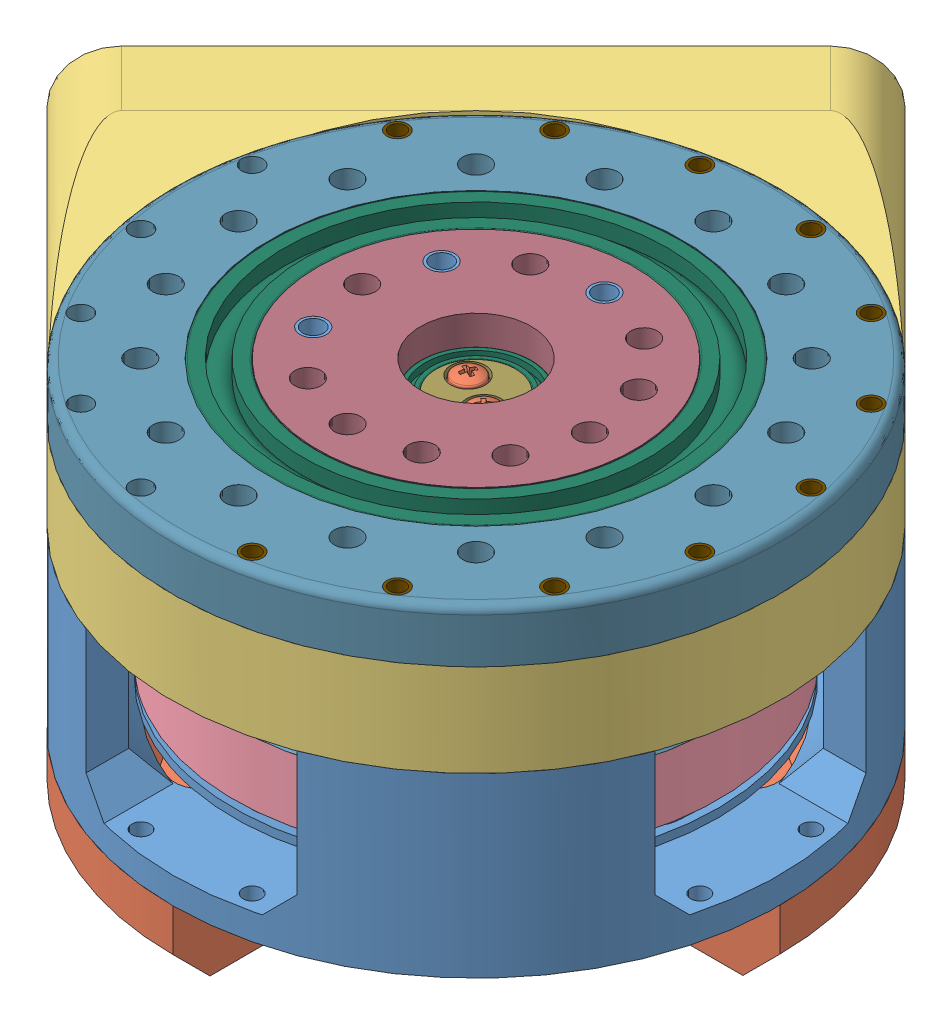
SolidWorks assembly Cycloidal_v2, configuration Default. Lengths in mm.
Overall size (173.24 87.5 173.24).
352 component instances, 93 part files, 142 mates.
Components (placement in the parent):
- motor-X83008S.stp-1: motor-X83008S.stp [Default] at (84.8609 89.8915 111.5645) x (-0.966627 0 -0.256188) z (0 -1 0) size (114.7 114.7 37.62)
  - base.stp-1: base.stp [Default] at (42.0794 12.0269 46.7342) size (91.6 91.6 15.61)
  - stator.stp-1: stator.stp [Default] at (42.0794 12.0269 33.1342) x (0.08493 -0.996387 0) z (0 0 1) size (83 83 8)
  - coil.stp-1: coil.stp [Default] at (39.5332 41.8984 37.1342) x (0.996387 0.08493 0) z (-0.08493 0.996387 0) size (4.4 10.2 10.5)
  - coil.stp-2: coil.stp [Default] at (34.3848 41.0025 37.1342) x (0.966502 0.256661 0) z (-0.256661 0.966502 0) size (4.4 10.2 10.5)
  - coil.stp-3: coil.stp [Default] at (29.4701 39.2261 37.1342) x (0.90725 0.420593 0) z (-0.420593 0.90725 0) size (4.4 10.2 10.5)
  - coil.stp-4: coil.stp [Default] at (24.9386 36.6233 37.1342) x (0.820431 0.571745 0) z (-0.571745 0.820431 0) size (4.4 10.2 10.5)
  - coil.stp-5: coil.stp [Default] at (20.9279 33.2732 37.1342) x (0.708685 0.705525 0) z (-0.705525 0.708685 0) size (4.4 10.2 10.5)
  - coil.stp-6: coil.stp [Default] at (17.5599 29.2775 37.1342) x (0.575405 0.817869 0) z (-0.817869 0.575405 0) size (4.4 10.2 10.5)
  - coil.stp-7: coil.stp [Default] at (14.9368 24.7576 37.1342) x (0.424642 0.905361 0) z (-0.905361 0.424642 0) size (4.4 10.2 10.5)
  - coil.stp-8: coil.stp [Default] at (13.1385 19.8509 37.1342) x (0.260976 0.965345 0) z (-0.965345 0.260976 0) size (4.4 10.2 10.5)
  - coil.stp-9: coil.stp [Default] at (12.2196 14.7066 37.1342) x (0.089381 0.995998 0) z (-0.995998 0.089381 0) size (4.4 10.2 10.5)
  - coil.stp-10: coil.stp [Default] at (12.2079 9.4807 37.1342) x (-0.08493 0.996387 0) z (-0.996387 -0.08493 0) size (4.4 10.2 10.5)
  - coil.stp-11: coil.stp [Default] at (13.1039 4.3323 37.1342) x (-0.256661 0.966502 0) z (-0.966502 -0.256661 0) size (4.4 10.2 10.5)
  - coil.stp-12: coil.stp [Default] at (14.8802 -0.5824 37.1342) x (-0.420593 0.90725 0) z (-0.90725 -0.420593 0) size (4.4 10.2 10.5)
  - coil.stp-13: coil.stp [Default] at (17.483 -5.1139 37.1342) x (-0.571745 0.820431 0) z (-0.820431 -0.571745 0) size (4.4 10.2 10.5)
  - coil.stp-14: coil.stp [Default] at (20.8332 -9.1246 37.1342) x (-0.705525 0.708685 0) z (-0.708685 -0.705525 0) size (4.4 10.2 10.5)
  - coil.stp-15: coil.stp [Default] at (24.8289 -12.4926 37.1342) x (-0.817869 0.575405 0) z (-0.575405 -0.817869 0) size (4.4 10.2 10.5)
  - coil.stp-16: coil.stp [Default] at (29.3487 -15.1157 37.1342) x (-0.905361 0.424642 0) z (-0.424642 -0.905361 0) size (4.4 10.2 10.5)
  - coil.stp-17: coil.stp [Default] at (34.2554 -16.914 37.1342) x (-0.965345 0.260976 0) z (-0.260976 -0.965345 0) size (4.4 10.2 10.5)
  - coil.stp-18: coil.stp [Default] at (39.3998 -17.8329 37.1342) x (-0.995998 0.089381 0) z (-0.089381 -0.995998 0) size (4.4 10.2 10.5)
  - coil.stp-19: coil.stp [Default] at (44.6256 -17.8446 37.1342) x (-0.996387 -0.08493 0) z (0.08493 -0.996387 0) size (4.4 10.2 10.5)
  - coil.stp-20: coil.stp [Default] at (49.7741 -16.9486 37.1342) x (-0.966502 -0.256661 0) z (0.256661 -0.966502 0) size (4.4 10.2 10.5)
  - coil.stp-21: coil.stp [Default] at (54.6887 -15.1723 37.1342) x (-0.90725 -0.420593 0) z (0.420593 -0.90725 0) size (4.4 10.2 10.5)
  - coil.stp-22: coil.stp [Default] at (59.2202 -12.5695 37.1342) x (-0.820431 -0.571745 0) z (0.571745 -0.820431 0) size (4.4 10.2 10.5)
  - coil.stp-23: coil.stp [Default] at (63.2309 -9.2193 37.1342) x (-0.708685 -0.705525 0) z (0.705525 -0.708685 0) size (4.4 10.2 10.5)
  - coil.stp-24: coil.stp [Default] at (66.599 -5.2236 37.1342) x (-0.575405 -0.817869 0) z (0.817869 -0.575405 0) size (4.4 10.2 10.5)
  - coil.stp-25: coil.stp [Default] at (69.222 -0.7038 37.1342) x (-0.424642 -0.905361 0) z (0.905361 -0.424642 0) size (4.4 10.2 10.5)
  - coil.stp-26: coil.stp [Default] at (71.0203 4.2029 37.1342) x (-0.260976 -0.965345 0) z (0.965345 -0.260976 0) size (4.4 10.2 10.5)
  - coil.stp-27: coil.stp [Default] at (71.9392 9.3473 37.1342) x (-0.089381 -0.995998 0) z (0.995998 -0.089381 0) size (4.4 10.2 10.5)
  - coil.stp-28: coil.stp [Default] at (71.9509 14.5731 37.1342) x (0.08493 -0.996387 0) z (0.996387 0.08493 0) size (4.4 10.2 10.5)
  - coil.stp-29: coil.stp [Default] at (71.055 19.7216 37.1342) x (0.256661 -0.966502 0) z (0.966502 0.256661 0) size (4.4 10.2 10.5)
  - coil.stp-30: coil.stp [Default] at (69.2786 24.6362 37.1342) x (0.420593 -0.90725 0) z (0.90725 0.420593 0) size (4.4 10.2 10.5)
  - coil.stp-31: coil.stp [Default] at (66.6758 29.1677 37.1342) x (0.571745 -0.820431 0) z (0.820431 0.571745 0) size (4.4 10.2 10.5)
  - coil.stp-32: coil.stp [Default] at (63.3257 33.1785 37.1342) x (0.705525 -0.708685 0) z (0.708685 0.705525 0) size (4.4 10.2 10.5)
  - coil.stp-33: coil.stp [Default] at (59.33 36.5465 37.1342) x (0.817869 -0.575405 0) z (0.575405 0.817869 0) size (4.4 10.2 10.5)
  - coil.stp-34: coil.stp [Default] at (54.8101 39.1695 37.1342) x (0.905361 -0.424642 0) z (0.424642 0.905361 0) size (4.4 10.2 10.5)
  - coil.stp-35: coil.stp [Default] at (49.9034 40.9678 37.1342) x (0.965345 -0.260976 0) z (0.260976 0.965345 0) size (4.4 10.2 10.5)
  - coil.stp-36: coil.stp [Default] at (44.759 41.8868 37.1342) x (0.995998 -0.089381 0) z (0.089381 0.995998 0) size (4.4 10.2 10.5)
  - rotor.stp-1: rotor.stp [Default] at (42.0794 12.0269 42.1342) x (-0.293442 0.955977 0) z (0 0 -1) size (91.8 91.8 12)
  - outrunner.stp-1: outrunner.stp [Default] at (42.0794 12.0269 30.1342) x (-0.254711 0.967017 0) z (-0.967017 -0.254711 0) size (91.8 17.01 91.8)
  - screw-mount.stp-1: screw-mount.stp [Default] at (38.1314 27.0157 27.1342) x (1 0 0) z (0 0 -1) size (7 7 6.5)
  - screw-mount.stp-2: screw-mount.stp [Default] at (27.0906 8.0789 27.1342) x (1 0 0) z (0 0 -1) size (7 7 6.5)
  - screw-mount.stp-3: screw-mount.stp [Default] at (57.0682 15.9749 27.1342) x (1 0 0) z (0 0 -1) size (7 7 6.5)
  - screw-mount.stp-4: screw-mount.stp [Default] at (46.0274 -2.9618 27.1342) x (1 0 0) z (0 0 -1) size (7 7 6.5)
  - 6702ZZ-bearing-15x21x4.stp-1: 6702ZZ-bearing-15x21x4.stp [Default] at (42.0794 12.0269 43.7342) x (1 0 0) z (0 -1 0) size (21 4 21)
  - 6702ZZ-bearing-15x21x4.stp-2: 6702ZZ-bearing-15x21x4.stp [Default] at (42.0794 12.0269 35.1342) x (1 0 0) z (0 1 0) size (21 4 21)
  - shaft.stp-1: shaft.stp [Default] at (42.0794 12.0269 20.1342) size (16 16 31.6)
  - fix-screw.stp-1: fix-screw.stp [Default] at (42.0794 12.0269 51.7342) x (1 0 0) z (0 0 -1) size (19.67 18.96 12.02)
- Base_Plate-1: Base_Plate [Default] at (47.267 69.7573 89.1587) x (0.869491 0 0.493949) z (-0.493949 0 0.869491) size (40 7 40)
- Eccentric_Shaft-1: Eccentric_Shaft [Default] at (31.2466 70.4165 88.8331) x (0.493949 0 -0.869491) z (0.869491 0 0.493949) size (20 15 17)
  - Eccentric_Shaft_bot-1: Eccentric_Shaft_bot [Default] at (7.6302 6.3409 14.0904) size (17 5 17)
  - Eccentric_Shaft_bot-2: Eccentric_Shaft_bot [Default] at (7.6302 11.3409 14.0904) x (-1 0 0) z (0 0 -1) size (17 5 17)
  - Eccentric_Shaft_top-1: Eccentric_Shaft_top [Default] at (7.6302 16.3409 14.0904) x (-1 0 0) z (0 0 -1) size (17 5 17)
- Output_Shaft-1: Output_Shaft [Default] at (47.267 87.2573 89.1587) x (-0.447203 0 -0.894433) z (0.894433 0 -0.447203) size (60 10 60)
- Cover-1: Cover [Default] at (47.267 87.2573 89.1587) x (0.707107 0 -0.707107) z (0.707107 0 0.707107) size (115 10.4 115)
- radial ball bearing_68_iso-39: radial ball bearing_68_iso [ISO 15 RBB - 1860 - 32,SI,NC,32_68] at (47.267 92.2573 89.1587) x (0 1 0) z (0 0 1) size (10 78 78)
- radial ball bearing_68_iso-40: radial ball bearing_68_iso [ISO 15 RBB - 1840 - 32,SI,NC,32_68] at (47.267 73.2573 89.1587) x (0 1 0) z (-0.019534 0 0.999809) size (7 52 52)
- m13_bearing-31: m13_bearing [Default] at (-10.7414 95.4081 67.0593) x (0.227678 0 0.973736) z (0.973736 0 -0.227678) size (13 16 13)
  - m6-1: m6 [Default] at (8.4921 2.5508 14.8914) size (6 16 6)
  - radial ball bearing_68_iso-1: radial ball bearing_68_iso [ISO 15 RBB - 286 - 10,SI,NC,10_68] at (8.4921 16.0508 14.8914) x (0 1 0) z (0 0 1) size (5 13 13)
  - radial ball bearing_68_iso-2: radial ball bearing_68_iso [ISO 15 RBB - 286 - 10,SI,NC,10_68] at (8.4921 11.0508 14.8914) x (0 1 0) z (0 0 1) size (5 13 13)
- m13_bearing-32: m13_bearing [Default] at (-14.1668 95.4081 84.2801) x (0.227678 0 0.973736) z (0.973736 0 -0.227678) size (13 16 13)
  - m6-1: m6 [Default] at (8.4921 2.5508 14.8914) size (6 16 6)
  - radial ball bearing_68_iso-1: radial ball bearing_68_iso [ISO 15 RBB - 286 - 10,SI,NC,10_68] at (8.4921 16.0508 14.8914) x (0 1 0) z (0 0 1) size (5 13 13)
  - radial ball bearing_68_iso-2: radial ball bearing_68_iso [ISO 15 RBB - 286 - 10,SI,NC,10_68] at (8.4921 11.0508 14.8914) x (0 1 0) z (0 0 1) size (5 13 13)
- m13_bearing-34: m13_bearing [Default] at (13.6125 95.5581 125.8547) x (0.227678 0 0.973736) z (0.973736 0 -0.227678) size (13 16 13)
  - m6-1: m6 [Default] at (8.4921 2.5508 14.8914) size (6 16 6)
  - radial ball bearing_68_iso-1: radial ball bearing_68_iso [ISO 15 RBB - 286 - 10,SI,NC,10_68] at (8.4921 16.0508 14.8914) x (0 1 0) z (0 0 1) size (5 13 13)
  - radial ball bearing_68_iso-2: radial ball bearing_68_iso [ISO 15 RBB - 286 - 10,SI,NC,10_68] at (8.4921 11.0508 14.8914) x (0 1 0) z (0 0 1) size (5 13 13)
- m13_bearing-35: m13_bearing [Default] at (-0.9866 95.4081 116.0999) x (0.227678 0 0.973736) z (0.973736 0 -0.227678) size (13 16 13)
  - m6-1: m6 [Default] at (8.4921 2.5508 14.8914) size (6 16 6)
  - radial ball bearing_68_iso-1: radial ball bearing_68_iso [ISO 15 RBB - 286 - 10,SI,NC,10_68] at (8.4921 16.0508 14.8914) x (0 1 0) z (0 0 1) size (5 13 13)
  - radial ball bearing_68_iso-2: radial ball bearing_68_iso [ISO 15 RBB - 286 - 10,SI,NC,10_68] at (8.4921 11.0508 14.8914) x (0 1 0) z (0 0 1) size (5 13 13)
- m13_bearing-36: m13_bearing [Default] at (-10.7414 95.5581 101.5009) x (0.227678 0 0.973736) z (0.973736 0 -0.227678) size (13 16 13)
  - m6-1: m6 [Default] at (8.4921 2.5508 14.8914) size (6 16 6)
  - radial ball bearing_68_iso-1: radial ball bearing_68_iso [ISO 15 RBB - 286 - 10,SI,NC,10_68] at (8.4921 16.0508 14.8914) x (0 1 0) z (0 0 1) size (5 13 13)
  - radial ball bearing_68_iso-2: radial ball bearing_68_iso [ISO 15 RBB - 286 - 10,SI,NC,10_68] at (8.4921 11.0508 14.8914) x (0 1 0) z (0 0 1) size (5 13 13)
- m13_bearing-1: m13_bearing [Default] at (-0.8801 95.4081 62.5627) x (0.736525 0 0.676411) z (0.676411 0 -0.736525) size (13 16 13)
  - m6-1: m6 [Default] at (8.4921 2.5508 14.8914) size (6 16 6)
  - radial ball bearing_68_iso-1: radial ball bearing_68_iso [ISO 15 RBB - 286 - 10,SI,NC,10_68] at (8.4921 16.0508 14.8914) x (0 1 0) z (0 0 1) size (5 13 13)
  - radial ball bearing_68_iso-2: radial ball bearing_68_iso [ISO 15 RBB - 286 - 10,SI,NC,10_68] at (8.4921 11.0508 14.8914) x (0 1 0) z (0 0 1) size (5 13 13)
- m13_bearing-2: m13_bearing [Default] at (48.6831 95.4081 124.0939) x (0.120271 0 0.992741) z (0.992741 0 -0.120271) size (13 16 13)
  - m6-1: m6 [Default] at (8.4921 2.5508 14.8914) size (6 16 6)
  - radial ball bearing_68_iso-1: radial ball bearing_68_iso [ISO 15 RBB - 286 - 10,SI,NC,10_68] at (8.4921 16.0508 14.8914) x (0 1 0) z (0 0 1) size (5 13 13)
  - radial ball bearing_68_iso-2: radial ball bearing_68_iso [ISO 15 RBB - 286 - 10,SI,NC,10_68] at (8.4921 11.0508 14.8914) x (0 1 0) z (0 0 1) size (5 13 13)
- m13_bearing-3: m13_bearing [Default] at (32.7832 95.4081 34.9886) x (-0.046141 0 0.998935) z (0.998935 0 0.046141) size (13 16 13)
  - m6-1: m6 [Default] at (8.4921 2.5508 14.8914) size (6 16 6)
  - radial ball bearing_68_iso-1: radial ball bearing_68_iso [ISO 15 RBB - 286 - 10,SI,NC,10_68] at (8.4921 16.0508 14.8914) x (0 1 0) z (0 0 1) size (5 13 13)
  - radial ball bearing_68_iso-2: radial ball bearing_68_iso [ISO 15 RBB - 286 - 10,SI,NC,10_68] at (8.4921 11.0508 14.8914) x (0 1 0) z (0 0 1) size (5 13 13)
- m13_bearing-4: m13_bearing [Default] at (77.1902 95.4081 81.0003) x (0.022268 0 0.999752) z (0.999752 0 -0.022268) size (13 16 13)
  - m6-1: m6 [Default] at (8.4921 2.5508 14.8914) size (6 16 6)
  - radial ball bearing_68_iso-1: radial ball bearing_68_iso [ISO 15 RBB - 286 - 10,SI,NC,10_68] at (8.4921 16.0508 14.8914) x (0 1 0) z (0 0 1) size (5 13 13)
  - radial ball bearing_68_iso-2: radial ball bearing_68_iso [ISO 15 RBB - 286 - 10,SI,NC,10_68] at (8.4921 11.0508 14.8914) x (0 1 0) z (0 0 1) size (5 13 13)
- m13_bearing-5: m13_bearing [Default] at (73.474 95.4081 98.7828) x (0.059133 0 0.99825) z (0.99825 0 -0.059133) size (13 16 13)
  - m6-1: m6 [Default] at (8.4921 2.5508 14.8914) size (6 16 6)
  - radial ball bearing_68_iso-1: radial ball bearing_68_iso [ISO 15 RBB - 286 - 10,SI,NC,10_68] at (8.4921 16.0508 14.8914) x (0 1 0) z (0 0 1) size (5 13 13)
  - radial ball bearing_68_iso-2: radial ball bearing_68_iso [ISO 15 RBB - 286 - 10,SI,NC,10_68] at (8.4921 11.0508 14.8914) x (0 1 0) z (0 0 1) size (5 13 13)
- m13_bearing-6: m13_bearing [Default] at (12.9248 95.4081 46.7315) x (0.451561 0 0.89224) z (0.89224 0 -0.451561) size (13 16 13)
  - m6-1: m6 [Default] at (8.4921 2.5508 14.8914) size (6 16 6)
  - radial ball bearing_68_iso-1: radial ball bearing_68_iso [ISO 15 RBB - 286 - 10,SI,NC,10_68] at (8.4921 16.0508 14.8914) x (0 1 0) z (0 0 1) size (5 13 13)
  - radial ball bearing_68_iso-2: radial ball bearing_68_iso [ISO 15 RBB - 286 - 10,SI,NC,10_68] at (8.4921 11.0508 14.8914) x (0 1 0) z (0 0 1) size (5 13 13)
- m13_bearing-7: m13_bearing [Default] at (56.6452 95.4081 32.3406) x (-0.545813 0 0.837907) z (0.837907 0 0.545813) size (13 16 13)
  - m6-1: m6 [Default] at (8.4921 2.5508 14.8914) size (6 16 6)
  - radial ball bearing_68_iso-1: radial ball bearing_68_iso [ISO 15 RBB - 286 - 10,SI,NC,10_68] at (8.4921 16.0508 14.8914) x (0 1 0) z (0 0 1) size (5 13 13)
  - radial ball bearing_68_iso-2: radial ball bearing_68_iso [ISO 15 RBB - 286 - 10,SI,NC,10_68] at (8.4921 11.0508 14.8914) x (0 1 0) z (0 0 1) size (5 13 13)
- m13_bearing-8: m13_bearing [Default] at (63.0373 95.4081 51.3153) x (0.158553 0 0.98735) z (0.98735 0 -0.158553) size (13 16 13)
  - m6-1: m6 [Default] at (8.4921 2.5508 14.8914) size (6 16 6)
  - radial ball bearing_68_iso-1: radial ball bearing_68_iso [ISO 15 RBB - 286 - 10,SI,NC,10_68] at (8.4921 16.0508 14.8914) x (0 1 0) z (0 0 1) size (5 13 13)
  - radial ball bearing_68_iso-2: radial ball bearing_68_iso [ISO 15 RBB - 286 - 10,SI,NC,10_68] at (8.4921 11.0508 14.8914) x (0 1 0) z (0 0 1) size (5 13 13)
- m13_bearing-9: m13_bearing [Default] at (83.8577 95.4081 55.5358) x (-0.687134 0 0.72653) z (0.72653 0 0.687134) size (13 16 13)
  - m6-1: m6 [Default] at (8.4921 2.5508 14.8914) size (6 16 6)
  - radial ball bearing_68_iso-1: radial ball bearing_68_iso [ISO 15 RBB - 286 - 10,SI,NC,10_68] at (8.4921 16.0508 14.8914) x (0 1 0) z (0 0 1) size (5 13 13)
  - radial ball bearing_68_iso-2: radial ball bearing_68_iso [ISO 15 RBB - 286 - 10,SI,NC,10_68] at (8.4921 11.0508 14.8914) x (0 1 0) z (0 0 1) size (5 13 13)
- m13_bearing-11: m13_bearing [Default] at (30.1977 95.4081 135.7424) x (0.57351 0 0.819198) z (0.819198 0 -0.57351) size (13 16 13)
  - m6-1: m6 [Default] at (8.4921 2.5508 14.8914) size (6 16 6)
  - radial ball bearing_68_iso-1: radial ball bearing_68_iso [ISO 15 RBB - 286 - 10,SI,NC,10_68] at (8.4921 16.0508 14.8914) x (0 1 0) z (0 0 1) size (5 13 13)
  - radial ball bearing_68_iso-2: radial ball bearing_68_iso [ISO 15 RBB - 286 - 10,SI,NC,10_68] at (8.4921 11.0508 14.8914) x (0 1 0) z (0 0 1) size (5 13 13)
- m13_bearing-12: m13_bearing [Default] at (62.8861 95.4081 115.3744) x (0.184178 0 0.982893) z (0.982893 0 -0.184178) size (13 16 13)
  - m6-1: m6 [Default] at (8.4921 2.5508 14.8914) size (6 16 6)
  - radial ball bearing_68_iso-1: radial ball bearing_68_iso [ISO 15 RBB - 286 - 10,SI,NC,10_68] at (8.4921 16.0508 14.8914) x (0 1 0) z (0 0 1) size (5 13 13)
  - radial ball bearing_68_iso-2: radial ball bearing_68_iso [ISO 15 RBB - 286 - 10,SI,NC,10_68] at (8.4921 11.0508 14.8914) x (0 1 0) z (0 0 1) size (5 13 13)
- socket button head screw_iso-2: socket button head screw_iso [ISO 7380 - M4 x 12 - 12N] at (47.267 67.4573 134.1587) x (0 1 0) z (-0.724148 0 0.689645) size (14.2 7.6 7.6)
- socket button head screw_iso-3: socket button head screw_iso [ISO 7380 - M4 x 12 - 12N] at (15.4472 67.4573 57.3389) x (0 1 0) z (-0.724148 0 0.689645) size (14.2 7.6 7.6)
- socket button head screw_iso-4: socket button head screw_iso [ISO 7380 - M4 x 12 - 12N] at (30.0462 67.4573 47.5841) x (0 1 0) z (-0.724148 0 0.689645) size (14.2 7.6 7.6)
- socket button head screw_iso-5: socket button head screw_iso [ISO 7380 - M4 x 12 - 12N] at (47.267 67.4573 44.1587) x (0 1 0) z (-0.724148 0 0.689645) size (14.2 7.6 7.6)
- socket button head screw_iso-6: socket button head screw_iso [ISO 7380 - M4 x 12 - 12N] at (64.4877 67.4573 47.5841) x (0 1 0) z (-0.724148 0 0.689645) size (14.2 7.6 7.6)
- socket button head screw_iso-8: socket button head screw_iso [ISO 7380 - M4 x 12 - 12N] at (88.8416 67.4573 71.9379) x (0 1 0) z (-0.724148 0 0.689645) size (14.2 7.6 7.6)
- socket button head screw_iso-9: socket button head screw_iso [ISO 7380 - M4 x 12 - 12N] at (92.267 67.4573 89.1587) x (0 1 0) z (-0.724148 0 0.689645) size (14.2 7.6 7.6)
- socket button head screw_iso-10: socket button head screw_iso [ISO 7380 - M4 x 12 - 12N] at (88.8416 67.4573 106.3794) x (0 1 0) z (-0.724148 0 0.689645) size (14.2 7.6 7.6)
- socket button head screw_iso-11: socket button head screw_iso [ISO 7380 - M4 x 12 - 12N] at (79.0868 67.4573 120.9785) x (0 1 0) z (-0.724148 0 0.689645) size (14.2 7.6 7.6)
- M3x4x4.2_brass_insert-2: M3x4x4.2_brass_insert [Default] at (2.3676 97.2573 59.1579) x (-0.680278 0 -0.732954) z (-0.732954 0 0.680278) size (4 4 4)
- M3x4x4.2_brass_insert-3: M3x4x4.2_brass_insert [Default] at (17.2662 97.2573 44.2593) x (-0.509546 0 -0.860444) z (-0.860444 0 0.509546) size (4 4 4)
- M3x4x4.2_brass_insert-6: M3x4x4.2_brass_insert [Default] at (77.2678 97.2573 44.2593) x (-0.680278 0 -0.732954) z (-0.732954 0 0.680278) size (4 4 4)
- M3x4x4.2_brass_insert-8: M3x4x4.2_brass_insert [Default] at (100.2294 93.2573 78.6238) x (-0.970393 0 0.241533) z (-0.241533 0 -0.970393) size (4 4 4)
- M3x4x4.2_brass_insert-14: M3x4x4.2_brass_insert [Default] at (36.7321 97.2573 36.1963) x (0.509546 0 0.860444) z (0.860444 0 -0.509546) size (4 4 4)
- M3x4x4.2_brass_insert-15: M3x4x4.2_brass_insert [Default] at (57.8019 93.2573 36.1963) x (0.897191 0 -0.441644) z (0.441644 0 0.897191) size (4 4 4)
- M3x4x4.2_brass_insert-16: M3x4x4.2_brass_insert [Default] at (92.1663 97.2573 59.1579) x (-0.680278 0 -0.732954) z (-0.732954 0 0.680278) size (4 4 4)
- M3x4x4.2_brass_insert-17: M3x4x4.2_brass_insert [Default] at (100.2294 97.2573 99.6935) x (0.680278 0 0.732954) z (0.732954 0 -0.680278) size (4 4 4)
- M3x4x4.2_brass_insert-19: M3x4x4.2_brass_insert [Default] at (92.1663 97.2573 119.1595) x (0.680278 0 0.732954) z (0.732954 0 -0.680278) size (4 4 4)
- M3x4x4.2_brass_insert-20: M3x4x4.2_brass_insert [Default] at (77.2678 97.2573 134.058) x (0.680278 0 0.732954) z (0.732954 0 -0.680278) size (4 4 4)
- M3x4x4.2_brass_insert-21: M3x4x4.2_brass_insert [Default] at (57.8019 97.2573 142.1211) x (0.680278 0 0.732954) z (0.732954 0 -0.680278) size (4 4 4)
- M4x6x5.5_brass_insert-47: M4x6x5.5_brass_insert [Default] at (5.6924 92.8573 71.9379) x (0.474598 0 0.880203) z (0 1 0) size (5 5 6)
- M4x6x5.5_brass_insert-48: M4x6x5.5_brass_insert [Default] at (2.267 92.8573 89.1587) x (0.260051 0 0.965595) z (0 1 0) size (5 5 6)
- M4x6x5.5_brass_insert-49: M4x6x5.5_brass_insert [Default] at (5.6924 87.0073 106.3794) x (-0.745833 0 0.666133) z (0 -1 0) size (5 5 6)
- M4x6x5.5_brass_insert-50: M4x6x5.5_brass_insert [Default] at (15.4472 86.8573 120.9785) x (-0.745833 0 0.666133) z (0 -1 0) size (5 5 6)
- M4x6x5.5_brass_insert-51: M4x6x5.5_brass_insert [Default] at (30.0462 87.0073 130.7332) x (0.260051 0 -0.965595) z (0 -1 0) size (5 5 6)
- M4x6x5.5_brass_insert-1: M4x6x5.5_brass_insert [Default] at (59.94 86.633 69.965) x (-0.745833 0 0.666133) z (0 -1 0) size (5 5 6)
- M4x6x5.5_brass_insert-6: M4x6x5.5_brass_insert [Default] at (24.3083 92.633 87.7803) x (0.252509 0 0.967595) z (0 1 0) size (5 5 6)
- M4x6x5.5_brass_insert-7: M4x6x5.5_brass_insert [Default] at (36.9813 92.633 68.5867) x (0.175665 0 0.98445) z (0 1 0) size (5 5 6)
- M4x6x5.5_brass_insert-9: M4x6x5.5_brass_insert [Default] at (48.6453 97.2573 66.2) x (0.260051 0 0.965595) z (0 1 0) size (5 5 6)
- M4x6x5.5_brass_insert-10: M4x6x5.5_brass_insert [Default] at (28.0734 97.2573 76.4857) x (0.009651 0 0.999953) z (0 1 0) size (5 5 6)
- M4x6x5.5_brass_insert-11: M4x6x5.5_brass_insert [Default] at (26.695 97.2573 99.4443) x (0.260051 0 0.965595) z (0 1 0) size (5 5 6)
- M4x6x5.5_brass_insert-20: M4x6x5.5_brass_insert [Default] at (64.4877 86.8573 130.7332) x (-0.745833 0 0.666133) z (0 -1 0) size (5 5 6)
- M4x6x5.5_brass_insert-21: M4x6x5.5_brass_insert [Default] at (47.267 86.8573 134.1587) x (-0.745833 0 0.666133) z (0 -1 0) size (5 5 6)
- M4x6x5.5_brass_insert-22: M4x6x5.5_brass_insert [Default] at (15.4472 86.8573 57.3389) x (0.623293 0 0.781988) z (0 -1 0) size (5 5 6)
- M4x6x5.5_brass_insert-23: M4x6x5.5_brass_insert [Default] at (30.0462 86.8573 47.5841) x (0.623293 0 0.781988) z (0 -1 0) size (5 5 6)
- M4x6x5.5_brass_insert-24: M4x6x5.5_brass_insert [Default] at (79.0868 86.8573 120.9785) x (0.541965 0 0.840401) z (0 -1 0) size (5 5 6)
- M4x6x5.5_brass_insert-25: M4x6x5.5_brass_insert [Default] at (88.8416 86.8573 106.3794) x (-0.745833 0 0.666133) z (0 -1 0) size (5 5 6)
- M4x6x5.5_brass_insert-26: M4x6x5.5_brass_insert [Default] at (92.267 86.8573 89.1587) x (-0.745833 0 0.666133) z (0 -1 0) size (5 5 6)
- M4x6x5.5_brass_insert-27: M4x6x5.5_brass_insert [Default] at (88.8416 86.8573 71.9379) x (-0.745833 0 0.666133) z (0 -1 0) size (5 5 6)
- M4x6x5.5_brass_insert-28: M4x6x5.5_brass_insert [Default] at (79.0868 92.8573 57.3389) x (0.260051 0 0.965595) z (0 1 0) size (5 5 6)
- M4x6x5.5_brass_insert-29: M4x6x5.5_brass_insert [Default] at (64.4877 86.8573 47.5841) x (-0.142939 0 0.989731) z (0 -1 0) size (5 5 6)
- M4x6x5.5_brass_insert-31: M4x6x5.5_brass_insert [Default] at (47.267 86.8573 44.1587) x (-0.220341 0 0.975423) z (0 -1 0) size (5 5 6)
- pan cross head_am-1: pan cross head_am [B18.6.7M - M3 x 0.5 x 20 Type I Cross Recessed PHMS --20N] at (50.745 92.6573 91.1345) x (0 -1 0) z (0.748822 0 0.662771) size (22.37 5.6 5.6)
- pan cross head_am-3: pan cross head_am [B18.6.7M - M3 x 0.5 x 20 Type I Cross Recessed PHMS --20N] at (43.789 92.6573 87.1829) x (0 -1 0) z (0.940321 0 0.340288) size (22.37 5.6 5.6)
- M3x4x4.2_brass_insert-22: M3x4x4.2_brass_insert [Default] at (50.745 69.7573 91.1345) x (0.984578 0 -0.174944) z (0.174944 0 0.984578) size (4 4 4)
- M3x4x4.2_brass_insert-23: M3x4x4.2_brass_insert [Default] at (43.789 69.7573 87.1829) x (0.984609 0 -0.174769) z (0.174769 0 0.984609) size (4 4 4)
- pan cross head_am-4: pan cross head_am [B18.6.7M - M3 x 0.5 x 10 Type I Cross Recessed PHMS --10N] at (33.7899 77.6573 81.5025) x (0 -1 0) z (0 0 1) size (12.37 5.6 5.6)
- pan cross head_am-5: pan cross head_am [B18.6.7M - M3 x 0.5 x 10 Type I Cross Recessed PHMS --10N] at (60.7441 77.6573 96.8149) x (0 -1 0) z (0 0 1) size (12.37 5.6 5.6)
- pan cross head_am-6: pan cross head_am [B18.6.7M - M3 x 0.5 x 10 Type I Cross Recessed PHMS --10N] at (39.6108 77.6573 102.6358) x (0 -1 0) z (0 0 1) size (12.37 5.6 5.6)
- pan cross head_am-7: pan cross head_am [B18.6.7M - M3 x 0.5 x 10 Type I Cross Recessed PHMS --10N] at (54.9232 77.6573 75.6816) x (0 -1 0) z (0 0 1) size (12.37 5.6 5.6)
- radial ball bearing_68_iso-44: radial ball bearing_68_iso [ISO 15 RBB - 1715 - 26,SI,NC,26_68] at (48.0079 84.7573 87.8544) x (0 1 0) z (-0.714953 0 -0.699173) size (4 21 21)
- radial ball bearing_68_iso-45: radial ball bearing_68_iso [ISO 15 RBB - 1715 - 26,SI,NC,26_68] at (47.267 89.7573 89.1587) x (0 1 0) z (0.999483 0 -0.032163) size (4 21 21)
- radial ball bearing_68_iso-46: radial ball bearing_68_iso [ISO 15 RBB - 1715 - 26,SI,NC,26_68] at (46.5261 79.7573 90.4629) x (0 1 0) z (0.000177 0 1) size (4 21 21)
- socket button head screw_iso-37: socket button head screw_iso [ISO 7380 - M4 x 12 - 12N] at (79.0868 67.4573 57.3389) x (0 1 0) z (-0.709975 0 0.704227) size (14.2 7.6 7.6)
- socket button head screw_iso-38: socket button head screw_iso [ISO 7380 - M4 x 12 - 12N] at (64.4877 67.4573 130.7332) x (0 1 0) z (-0.724148 0 0.689645) size (14.2 7.6 7.6)
- foc-motor-controller.step-1: foc-motor-controller.step [Default] at (47.267 33.7573 89.1587) x (-0.707107 0 -0.707107) z (0 -1 0) size (57.23 50 8.13)
  - RTA0040B.step-1: RTA0040B.step [Default] at (12.5014 -1.6986 1.595) x (-0.707107 -0.707107 0) z (0 0 1) size (6 6 1)
    - FRAME.step-1: FRAME.step [Default] x (1 0 0) z (0 -1 0) size (6 0.2 6)
      - SOLID.step-1: SOLID.step [Default] at origin size (0.4 0.2 0.22)
      - SOLID-0.step-1: SOLID-0.step [Default] at origin size (0.4 0.2 0.22)
      - SOLID-1.step-1: SOLID-1.step [Default] at origin size (0.4 0.2 0.22)
      - SOLID-2.step-1: SOLID-2.step [Default] at origin size (0.4 0.2 0.22)
      - SOLID-3.step-1: SOLID-3.step [Default] at origin size (0.4 0.2 0.22)
      - SOLID-4.step-1: SOLID-4.step [Default] at origin size (0.4 0.2 0.22)
      - SOLID-5.step-1: SOLID-5.step [Default] at origin size (0.4 0.2 0.22)
      - SOLID-6.step-1: SOLID-6.step [Default] at origin size (0.4 0.2 0.22)
      - SOLID-7.step-1: SOLID-7.step [Default] at origin size (0.4 0.2 0.22)
      - SOLID-8.step-1: SOLID-8.step [Default] at origin size (0.4 0.2 0.22)
      - SOLID-9.step-1: SOLID-9.step [Default] at origin size (0.22 0.2 0.4)
      - SOLID-10.step-1: SOLID-10.step [Default] at origin size (0.22 0.2 0.4)
      - SOLID-11.step-1: SOLID-11.step [Default] at origin size (0.22 0.2 0.4)
      - SOLID-12.step-1: SOLID-12.step [Default] at origin size (0.22 0.2 0.4)
      - SOLID-13.step-1: SOLID-13.step [Default] at origin size (0.22 0.2 0.4)
      - SOLID-14.step-1: SOLID-14.step [Default] at origin size (0.22 0.2 0.4)
      - SOLID-15.step-1: SOLID-15.step [Default] at origin size (0.22 0.2 0.4)
      - SOLID-16.step-1: SOLID-16.step [Default] at origin size (0.22 0.2 0.4)
      - SOLID-17.step-1: SOLID-17.step [Default] at origin size (4.15 0.2 4.15)
      - SOLID-18.step-1: SOLID-18.step [Default] at origin size (0.28 0.1 0.28)
      - SOLID-19.step-1: SOLID-19.step [Default] at origin size (0.28 0.1 0.28)
      - SOLID-20.step-1: SOLID-20.step [Default] at origin size (0.28 0.1 0.28)
      - SOLID-21.step-1: SOLID-21.step [Default] at origin size (0.28 0.1 0.28)
      - SOLID-22.step-1: SOLID-22.step [Default] at origin size (0.4 0.2 0.22)
      - SOLID-23.step-1: SOLID-23.step [Default] at origin size (0.4 0.2 0.22)
      - SOLID-24.step-1: SOLID-24.step [Default] at origin size (0.4 0.2 0.22)
      - SOLID-25.step-1: SOLID-25.step [Default] at origin size (0.4 0.2 0.22)
      - SOLID-26.step-1: SOLID-26.step [Default] at origin size (0.4 0.2 0.22)
      - SOLID-27.step-1: SOLID-27.step [Default] at origin size (0.4 0.2 0.22)
      - SOLID-28.step-1: SOLID-28.step [Default] at origin size (0.4 0.2 0.22)
      - SOLID-29.step-1: SOLID-29.step [Default] at origin size (0.4 0.2 0.22)
      - SOLID-30.step-1: SOLID-30.step [Default] at origin size (0.4 0.2 0.22)
      - SOLID-31.step-1: SOLID-31.step [Default] at origin size (0.4 0.2 0.22)
      - SOLID-32.step-1: SOLID-32.step [Default] at origin size (0.22 0.2 0.4)
      - SOLID-33.step-1: SOLID-33.step [Default] at origin size (0.22 0.2 0.4)
      - SOLID-34.step-1: SOLID-34.step [Default] at origin size (0.22 0.2 0.4)
      - SOLID-35.step-1: SOLID-35.step [Default] at origin size (0.22 0.2 0.4)
      - SOLID-36.step-1: SOLID-36.step [Default] at origin size (0.22 0.2 0.4)
      - SOLID-37.step-1: SOLID-37.step [Default] at origin size (0.22 0.2 0.4)
      - SOLID-38.step-1: SOLID-38.step [Default] at origin size (0.22 0.2 0.4)
      - SOLID-39.step-1: SOLID-39.step [Default] at origin size (0.22 0.2 0.4)
      - SOLID-40.step-1: SOLID-40.step [Default] at origin size (0.22 0.2 0.4)
      - SOLID-41.step-1: SOLID-41.step [Default] at origin size (0.22 0.2 0.4)
      - SOLID-42.step-1: SOLID-42.step [Default] at origin size (0.22 0.2 0.4)
      - SOLID-43.step-1: SOLID-43.step [Default] at origin size (0.22 0.2 0.4)
    - BODY.step-1: BODY.step [Default] at (0 0 0.025) x (1 0 0) z (0 -1 0) size (6 0.97 6)
  - Resonator_SMD_Murata_CSTxExxV-3Pin_3.0x1.1mm.step-1: Resonator_SMD_Murata_CSTxExxV-3Pin_3.0x1.1mm.step [Default] at (1.8 -7 1.595) x (0 1 0) z (0 0 1) size (3.2 1.35 0.9)
  - C_0603_1608Metric.step-1: C_0603_1608Metric.step [Default] at (6.2 -16.8 1.595) x (0 -1 0) z (0 0 1) size (1.6 0.8 0.8)
  - R_0603_1608Metric.step-1: R_0603_1608Metric.step [Default] at (11.8 -7.375 1.595) x (0 1 0) z (0 0 1) size (1.6 0.8 0.45)
  - R_0603_1608Metric.step-2: R_0603_1608Metric.step [Default] at (13.8 -16.8 1.595) x (0 1 0) z (0 0 1) size (1.6 0.8 0.45)
  - R_0603_1608Metric.step-3: R_0603_1608Metric.step [Default] at (18.1 -5.36 1.595) size (1.6 0.8 0.45)
  - C_0603_1608Metric.step-2: C_0603_1608Metric.step [Default] at (2.6 -0.5 1.595) x (0 -1 0) z (0 0 1) size (1.6 0.8 0.8)
  - R_0603_1608Metric.step-4: R_0603_1608Metric.step [Default] at (14.6 -11.3 1.595) x (0 1 0) z (0 0 1) size (1.6 0.8 0.45)
  - L_APV_ANR4020.step-1: L_APV_ANR4020.step [Default] at (22.3 -13.7 1.595) x (0 -1 0) z (0 0 1) size (4.02 4 2)
  - C_0603_1608Metric.step-3: C_0603_1608Metric.step [Default] at (0.3 -12.6 1.595) x (-1 0 0) z (0 0 1) size (1.6 0.8 0.8)
  - C_1206_3216Metric.step-1: C_1206_3216Metric.step [Default] at (15.7 11 1.595) x (0 1 0) z (0 0 1) size (3.2 1.6 1.6)
  - C_0603_1608Metric.step-4: C_0603_1608Metric.step [Default] at (0.3 -9.6 1.595) size (1.6 0.8 0.8)
  - R_0603_1608Metric.step-5: R_0603_1608Metric.step [Default] at (12.3 -16.8 1.595) x (0 1 0) z (0 0 1) size (1.6 0.8 0.45)
  - C_0603_1608Metric.step-5: C_0603_1608Metric.step [Default] at (-0.3 -16.6 1.595) x (0 1 0) z (0 0 1) size (1.6 0.8 0.8)
  - R_0603_1608Metric.step-6: R_0603_1608Metric.step [Default] at (10.9 4.1 1.595) size (1.6 0.8 0.45)
  - C_1206_3216Metric.step-2: C_1206_3216Metric.step [Default] at (6.3 11 1.595) x (0 1 0) z (0 0 1) size (3.2 1.6 1.6)
  - XT30PW_2_2_-M.G.B.step-1: XT30PW_2_2_-M.G.B.step [Default] at (-20.5 9.5 1.595) x (0 -1 0) z (-1 0 0) size (15.5 7.1 12.53)
  - R_0603_1608Metric.step-7: R_0603_1608Metric.step [Default] at (0.3 -11.1 1.595) size (1.6 0.8 0.45)
  - C_0603_1608Metric.step-6: C_0603_1608Metric.step [Default] at (19 -0.4 1.595) x (-0.707107 -0.707107 0) z (0 0 1) size (1.6 0.8 0.8)
  - C_1206_3216Metric.step-3: C_1206_3216Metric.step [Default] at (13.3 11 1.595) x (0 1 0) z (0 0 1) size (3.2 1.6 1.6)
  - R_0603_1608Metric.step-8: R_0603_1608Metric.step [Default] at (10.2 -7.375 1.595) x (0 -1 0) z (0 0 1) size (1.6 0.8 0.45)
  - JST_GH_SM08B-GHS-TB_1x08-1MP_P1.25mm_Horizontal.step-1: JST_GH_SM08B-GHS-TB_1x08-1MP_P1.25mm_Horizontal.step [Default] at (10 -22 1.595) size (13.25 4.95 4.25)
  - C_1206_3216Metric.step-4: C_1206_3216Metric.step [Default] at (-12.3 11 1.595) x (0 1 0) z (0 0 1) size (3.2 1.6 1.6)
  - JST_GH_SM06B-GHS-TB_1x06-1MP_P1.25mm_Horizontal.step-1: JST_GH_SM06B-GHS-TB_1x06-1MP_P1.25mm_Horizontal.step [Default] at (-4.3 -22 1.595) size (10.75 4.95 4.25)
  - C_0603_1608Metric.step-7: C_0603_1608Metric.step [Default] at (7.3 -4.5 1.595) x (-1 0 0) z (0 0 1) size (1.6 0.8 0.8)
  - R_0603_1608Metric.step-9: R_0603_1608Metric.step [Default] at (18.1 -3.86 1.595) x (-1 0 0) z (0 0 1) size (1.6 0.8 0.45)
  - C_1206_3216Metric.step-5: C_1206_3216Metric.step [Default] at (22.6794 -1.2206 1.595) x (0.707107 -0.707107 0) z (0 0 1) size (3.2 1.6 1.6)
  - R_Array_Convex_4x0402.step-1: R_Array_Convex_4x0402.step [Default] at (6.8 -2.5 1.595) size (1 2 0.35)
  - R_0603_1608Metric.step-10: R_0603_1608Metric.step [Default] at (7.7 -16.8 1.595) x (0 -1 0) z (0 0 1) size (1.6 0.8 0.45)
  - C_1206_3216Metric.step-6: C_1206_3216Metric.step [Default] at (8.7 11 1.595) x (0 1 0) z (0 0 1) size (3.2 1.6 1.6)
  - C_0603_1608Metric.step-8: C_0603_1608Metric.step [Default] at (16.1 -11.3 1.595) x (0 1 0) z (0 0 1) size (1.6 0.8 0.8)
  - SOT-23-5.step-1: SOT-23-5.step [Default] at (-3.1 -16.6 1.595) x (-1 0 0) z (0 0 1) size (2.8 2.9 1.55)
  - C_0603_1608Metric.step-9: C_0603_1608Metric.step [Default] at (17.8 -13.6 1.595) size (1.6 0.8 0.8)
  - R_0603_1608Metric.step-11: R_0603_1608Metric.step [Default] at (-11.5 -20.3875 1.595) x (0 -1 0) z (0 0 1) size (1.6 0.8 0.45)
  - C_0603_1608Metric.step-10: C_0603_1608Metric.step [Default] at (-12.4 2.3 1.595) x (0 1 0) z (0 0 1) size (1.6 0.8 0.8)
  - C_1206_3216Metric.step-7: C_1206_3216Metric.step [Default] at (18 11 1.595) x (0 1 0) z (0 0 1) size (3.2 1.6 1.6)
  - R_0603_1608Metric.step-12: R_0603_1608Metric.step [Default] at (-10.8105 -14.9971 1.595) x (-1 0 0) z (0 0 1) size (1.6 0.8 0.45)
  - C_0603_1608Metric.step-11: C_0603_1608Metric.step [Default] at (-13.8 -9.4 1.595) x (-1 0 0) z (0 0 1) size (1.6 0.8 0.8)
  - R_0603_1608Metric.step-13: R_0603_1608Metric.step [Default] at (-23.15 -14.5 1.595) x (-1 0 0) z (0 0 1) size (1.6 0.8 0.45)
  - C_0603_1608Metric.step-12: C_0603_1608Metric.step [Default] at (1.1 -0.2 1.595) x (0 1 0) z (0 0 1) size (1.6 0.8 0.8)
  - D_0805_2012Metric.step-1: D_0805_2012Metric.step [Default] at (22.9 -9.6 1.595) x (0 1 0) z (0 0 1) size (2 1.27 0.8)
  - C_0603_1608Metric.step-13: C_0603_1608Metric.step [Default] at (-7.8 3.775 1.595) x (0 -1 0) z (0 0 1) size (1.6 0.8 0.8)
  - R_0603_1608Metric.step-14: R_0603_1608Metric.step [Default] at (-6.4 -12.825 1.595) x (0 1 0) z (0 0 1) size (1.6 0.8 0.45)
  - L_0603_1608Metric.step-1: L_0603_1608Metric.step [Default] at (-10.1 3 1.595) size (1.6 0.8 0.8)
  - C_0603_1608Metric.step-14: C_0603_1608Metric.step [Default] at (17.9 0.7 1.595) x (-0.707107 -0.707107 0) z (0 0 1) size (1.6 0.8 0.8)
  - HVSSOP-10.step-1: HVSSOP-10.step [Default] at (18.6 -9.6 1.595) x (0 -1 0) z (-1 0 0) size (4.9 1.1 3)
  - C_0603_1608Metric.step-15: C_0603_1608Metric.step [Default] at (7.9 4.1 1.595) x (-1 0 0) z (0 0 1) size (1.6 0.8 0.8)
  - C_0603_1608Metric.step-16: C_0603_1608Metric.step [Default] at (21.1 -9.6 1.595) x (0 -1 0) z (0 0 1) size (1.6 0.8 0.8)
  - R_0603_1608Metric.step-15: R_0603_1608Metric.step [Default] at (-10.8105 -11.9971 1.595) x (-1 0 0) z (0 0 1) size (1.6 0.8 0.45)
  - R_0603_1608Metric.step-16: R_0603_1608Metric.step [Default] at (-18.2 -17.4 1.595) size (1.6 0.8 0.45)
  - C_1206_3216Metric.step-8: C_1206_3216Metric.step [Default] at (-3 11 1.595) x (0 1 0) z (0 0 1) size (3.2 1.6 1.6)
  - R_0603_1608Metric.step-17: R_0603_1608Metric.step [Default] at (-16.9 -20.4 1.595) x (0 -1 0) z (0 0 1) size (1.6 0.8 0.45)
  - R_0603_1608Metric.step-18: R_0603_1608Metric.step [Default] at (-13.3 -20.3875 1.595) x (0 -1 0) z (0 0 1) size (1.6 0.8 0.45)
  - R_0603_1608Metric.step-19: R_0603_1608Metric.step [Default] at (-15.1 -20.3875 1.595) x (0 -1 0) z (0 0 1) size (1.6 0.8 0.45)
  - C_0603_1608Metric.step-17: C_0603_1608Metric.step [Default] at (15.5 -14.4 1.595) x (0 -1 0) z (0 0 1) size (1.6 0.8 0.8)
  - LED_0603_1608Metric.step-1: LED_0603_1608Metric.step [Default] at (-11.5 -23.3875 1.595) x (0 1 0) z (0 0 1) size (1.6 0.8 1.1)
  - C_0805_2012Metric.step-1: C_0805_2012Metric.step [Default] at (19.95 -17 1.595) size (2 1.25 1.25)
  - D_SMB.step-1: D_SMB.step [Default] at (-16.5 11.208 1.595) x (0 -1 0) z (0 0 1) size (5.3 3.55 2.15)
  - C_1206_3216Metric.step-9: C_1206_3216Metric.step [Default] at (-5.3 11 1.595) x (0 1 0) z (0 0 1) size (3.2 1.6 1.6)
  - XT30PW_2_2_-M.G.B.step-2: XT30PW_2_2_-M.G.B.step [Default] at (-20.5 -6.5 1.595) x (0 -1 0) z (-1 0 0) size (15.5 7.1 12.53)
  - C_1206_3216Metric.step-10: C_1206_3216Metric.step [Default] at (1.7 11 1.595) x (0 1 0) z (0 0 1) size (3.2 1.6 1.6)
  - C_1206_3216Metric.step-11: C_1206_3216Metric.step [Default] at (11 11 1.595) x (0 1 0) z (0 0 1) size (3.2 1.6 1.6)
  - C_0603_1608Metric.step-18: C_0603_1608Metric.step [Default] at (-6.3 3.775 1.595) x (0 -1 0) z (0 0 1) size (1.6 0.8 0.8)
  - C_0603_1608Metric.step-19: C_0603_1608Metric.step [Default] at (16.8686 1.7314 1.595) x (0.707107 0.707107 0) z (0 0 1) size (1.6 0.8 0.8)
  - C_0603_1608Metric.step-20: C_0603_1608Metric.step [Default] at (-15.0105 -11.1 1.595) size (1.6 0.8 0.8)
  - C_1206_3216Metric.step-12: C_1206_3216Metric.step [Default] at (-7.7 11 1.595) x (0 1 0) z (0 0 1) size (3.2 1.6 1.6)
  - C_0603_1608Metric.step-21: C_0603_1608Metric.step [Default] at (-18.2 -15.8 1.595) size (1.6 0.8 0.8)
  - C_0603_1608Metric.step-22: C_0603_1608Metric.step [Default] at (-2.1 -11.3 1.595) x (0 -1 0) z (0 0 1) size (1.6 0.8 0.8)
  - C_0603_1608Metric.step-23: C_0603_1608Metric.step [Default] at (-10.8105 -13.4971 1.595) size (1.6 0.8 0.8)
  - C_1206_3216Metric.step-13: C_1206_3216Metric.step [Default] at (4 11 1.595) x (0 1 0) z (0 0 1) size (3.2 1.6 1.6)
  - R_0603_1608Metric.step-20: R_0603_1608Metric.step [Default] at (16 -17.8 1.595) x (0 1 0) z (0 0 1) size (1.6 0.8 0.45)
  - Texas_S-PVSON-N8.step-1: Texas_S-PVSON-N8.step [Default] at (-14.4105 -13.7 1.595) x (-1 0 0) z (0 0 1) size (3 2.98 0.92)
  - C_1206_3216Metric.step-14: C_1206_3216Metric.step [Default] at (21 -2.9 1.595) x (0.707107 -0.707107 0) z (0 0 1) size (3.2 1.6 1.6)
  - C_0603_1608Metric.step-24: C_0603_1608Metric.step [Default] at (-5.9 -16.6 1.595) x (0 1 0) z (0 0 1) size (1.6 0.8 0.8)
  - C_0603_1608Metric.step-25: C_0603_1608Metric.step [Default] at (-3.1 -14.1 1.595) size (1.6 0.8 0.8)
  - R_0603_1608Metric.step-21: R_0603_1608Metric.step [Default] at (7.2 -7.375 1.595) x (0 -1 0) z (0 0 1) size (1.6 0.8 0.45)
  - C_1206_3216Metric.step-15: C_1206_3216Metric.step [Default] at (-0.7 11 1.595) x (0 1 0) z (0 0 1) size (3.2 1.6 1.6)
  - LQFP-64_10x10mm_P0.5mm.step-1: LQFP-64_10x10mm_P0.5mm.step [Default] at (-7 -4.5 1.595) x (-1 0 0) z (0 0 1) size (12 12 1.5)
  - C_0805_2012Metric.step-2: C_0805_2012Metric.step [Default] at (23.35 -17 1.595) x (-1 0 0) z (0 0 1) size (2 1.25 1.25)
  - C_0603_1608Metric.step-26: C_0603_1608Metric.step [Default] at (10.8 -16.8 1.595) x (0 -1 0) z (0 0 1) size (1.6 0.8 0.8)
  - R_0603_1608Metric.step-22: R_0603_1608Metric.step [Default] at (17.5 -17.8 1.595) x (0 -1 0) z (0 0 1) size (1.6 0.8 0.45)
  - C_1206_3216Metric.step-16: C_1206_3216Metric.step [Default] at (20.3 11 1.595) x (0 1 0) z (0 0 1) size (3.2 1.6 1.6)
  - R_0603_1608Metric.step-23: R_0603_1608Metric.step [Default] at (9.2 -16.8 1.595) x (0 -1 0) z (0 0 1) size (1.6 0.8 0.45)
  - C_1206_3216Metric.step-17: C_1206_3216Metric.step [Default] at (-10 11 1.595) x (0 1 0) z (0 0 1) size (3.2 1.6 1.6)
  - R_0603_1608Metric.step-24: R_0603_1608Metric.step [Default] at (17.8 -15.2 1.595) size (1.6 0.8 0.45)
  - C_1206_3216Metric.step-18: C_1206_3216Metric.step [Default] at (19.9 2.6 1.595) x (-0.707107 0.707107 0) z (0 0 1) size (3.2 1.6 1.6)
  - C_0603_1608Metric.step-27: C_0603_1608Metric.step [Default] at (13.4 -7.375 1.595) x (0 -1 0) z (0 0 1) size (1.6 0.8 0.8)
  - R_0603_1608Metric.step-25: R_0603_1608Metric.step [Default] at (8.7 -7.375 1.595) x (0 -1 0) z (0 0 1) size (1.6 0.8 0.45)
  - PQFN-8-EP_6x5mm_P1.27mm_Generic.step-1: PQFN-8-EP_6x5mm_P1.27mm_Generic.step [Default] at (4.9 14.4 -0.085) x (0 1 0) z (0 0 -1) size (6.15 5.15 1.09)
  - C_0805_2012Metric.step-3: C_0805_2012Metric.step [Default] at (-3 8.9 -0.085) x (0 1 0) z (0 0 -1) size (2 1.25 1.25)
  - C_0603_1608Metric.step-28: C_0603_1608Metric.step [Default] at (1.5 -4.3 -0.085) x (0 1 0) z (0 0 -1) size (1.6 0.8 0.8)
  - R_2512_6332Metric.step-1: R_2512_6332Metric.step [Default] at (2.1 8.6 -0.085) x (-1 0 0) z (0 0 -1) size (6.3 3.2 0.6)
  - C_0805_2012Metric.step-4: C_0805_2012Metric.step [Default] at (18.8 8.9 -0.085) x (0 1 0) z (0 0 -1) size (2 1.25 1.25)
  - C_0805_2012Metric.step-5: C_0805_2012Metric.step [Default] at (-5.2 8.901 -0.085) x (0 1 0) z (0 0 -1) size (2 1.25 1.25)
  - PQFN-8-EP_6x5mm_P1.27mm_Generic.step-2: PQFN-8-EP_6x5mm_P1.27mm_Generic.step [Default] at (16.9 14.6 -0.085) x (0 -1 0) z (0 0 -1) size (6.15 5.15 1.09)
  - PQFN-8-EP_6x5mm_P1.27mm_Generic.step-3: PQFN-8-EP_6x5mm_P1.27mm_Generic.step [Default] at (-1.1 14.6 -0.085) x (0 -1 0) z (0 0 -1) size (6.15 5.15 1.09)
  - R_0603_1608Metric.step-26: R_0603_1608Metric.step [Default] at (8.2 8.8 -0.085) x (0 1 0) z (0 0 -1) size (1.6 0.8 0.45)
  - R_2512_6332Metric.step-2: R_2512_6332Metric.step [Default] at (-10.3 8.601 -0.085) x (1 0 0) z (0 0 -1) size (6.3 3.2 0.6)
  - TSSOP-16_4.4x5mm_P0.65mm.step-1: TSSOP-16_4.4x5mm_P0.65mm.step [Default] at (0 0 -0.085) x (-1 0 0) z (0 0 -1) size (6.4 5 1.1)
  - C_0603_1608Metric.step-29: C_0603_1608Metric.step [Default] at (0 -4.25 -0.085) x (0 1 0) z (0 0 -1) size (1.6 0.8 0.8)
  - PQFN-8-EP_6x5mm_P1.27mm_Generic.step-4: PQFN-8-EP_6x5mm_P1.27mm_Generic.step [Default] at (10.9 14.4 -0.085) x (0 1 0) z (0 0 -1) size (6.15 5.15 1.09)
  - R_2512_6332Metric.step-3: R_2512_6332Metric.step [Default] at (13.7 8.6 -0.085) x (1 0 0) z (0 0 -1) size (6.3 3.2 0.6)
  - PQFN-8-EP_6x5mm_P1.27mm_Generic.step-5: PQFN-8-EP_6x5mm_P1.27mm_Generic.step [Default] at (-13.1 14.401 -0.085) x (0 1 0) z (0 0 -1) size (6.15 5.15 1.09)
  - C_0603_1608Metric.step-30: C_0603_1608Metric.step [Default] at (-1.5 -4.3 -0.085) x (0 -1 0) z (0 0 -1) size (1.6 0.8 0.8)
  - PQFN-8-EP_6x5mm_P1.27mm_Generic.step-6: PQFN-8-EP_6x5mm_P1.27mm_Generic.step [Default] at (-7.1 14.601 -0.085) x (0 -1 0) z (0 0 -1) size (6.15 5.15 1.09)
  - foc-motor-controller_PCB.step-1: foc-motor-controller_PCB.step [Default] at origin size (50 50 1.51)
